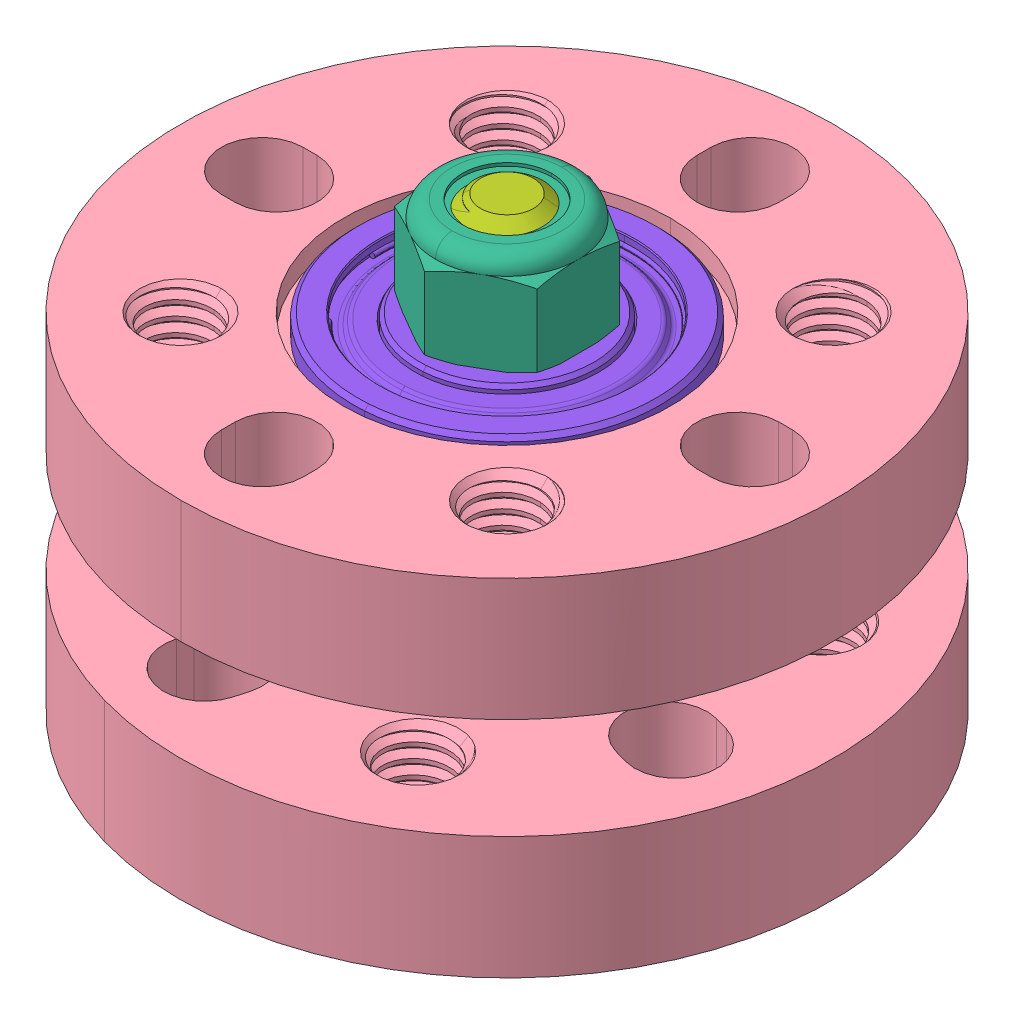
SolidWorks assembly 1608-0001-0001 assembly, configuration Default. Lengths in mm.
Overall size (39.45 26.01 39.45).
22 component instances, 9 part files, 0 mates.
Components (placement in the parent):
- 1608-0001-0001 assembly.STEP-1: 1608-0001-0001 assembly.STEP [Default] at origin size (39.45 26.01 39.45)
  - 1613-0516-0008 assembly.STEP-1: 1613-0516-0008 assembly.STEP [Default] at (13.2242 -21.7608 12.1381) x (0.966093 0 0.258196) z (-0.258196 0 0.966093) size (17.83 4.96 17.83)
    - 1613-0516-0008 carriage.STEP-1: 1613-0516-0008 carriage.STEP [Default] at (-23.0253 -4.8501 14.8236) size (15.72 1.83 15.72)
    - 1613-0516-0008 ball.STEP-1: 1613-0516-0008 ball.STEP [Default] at (-28.8255 -3.9351 16.4353) size (3 3 3)
    - 1613-0516-0008 ball.STEP-2: 1613-0516-0008 ball.STEP [Default] at (-26.4325 -3.9351 19.7866) x (0.766044 0 -0.642788) z (0.642788 0 0.766044) size (3 3 3)
    - 1613-0516-0008 ball.STEP-3: 1613-0516-0008 ball.STEP [Default] at (-22.4452 -3.9351 20.8156) x (0.173648 0 -0.984808) z (0.984808 0 0.173648) size (3 3 3)
    - 1613-0516-0008 ball.STEP-4: 1613-0516-0008 ball.STEP [Default] at (-18.7293 -3.9351 19.0408) x (-0.5 0 -0.866025) z (0.866025 0 -0.5) size (3 3 3)
    - 1613-0516-0008 ball.STEP-5: 1613-0516-0008 ball.STEP [Default] at (-17.0236 -3.9351 15.2928) x (-0.939693 0 -0.34202) z (0.34202 0 -0.939693) size (3 3 3)
    - 1613-0516-0008 ball.STEP-6: 1613-0516-0008 ball.STEP [Default] at (-18.1261 -3.9351 11.3252) x (-0.939693 0 0.34202) z (-0.34202 0 -0.939693) size (3 3 3)
    - 1613-0516-0008 ball.STEP-7: 1613-0516-0008 ball.STEP [Default] at (-21.521 -3.9351 8.9945) x (-0.5 0 0.866025) z (-0.866025 0 -0.5) size (3 3 3)
    - 1613-0516-0008 ball.STEP-8: 1613-0516-0008 ball.STEP [Default] at (-25.6197 -3.9351 9.3913) x (0.173648 0 0.984808) z (-0.984808 0 0.173648) size (3 3 3)
    - 1613-0516-0008 ball.STEP-9: 1613-0516-0008 ball.STEP [Default] at (-28.5045 -3.9351 12.3299) x (0.766044 0 0.642788) z (-0.642788 0 0.766044) size (3 3 3)
    - 1613-0516-0008 washer.STEP-1: 1613-0516-0008 washer.STEP [Default] at (-23.0253 -6.4151 14.8236) size (16 1.28 16)
    - 1613-0516-0008 washer.STEP-2: 1613-0516-0008 washer.STEP [Default] at (-23.0253 -1.4551 14.8236) x (0.992523 0 -0.12206) z (-0.12206 0 -0.992523) size (16 1.28 16)
  - 1504-0032-0060.STEP-1: 1504-0032-0060.STEP [Default] at (-12.8477 -20.2159 20.514) size (31.95 6.01 31.95)
  - 1504-0032-0060.STEP-2: 1504-0032-0060.STEP [Default] at (-12.8477 -31.1759 20.514) x (-0.962134 0 -0.272576) z (-0.272576 0 0.962134) size (31.95 6.01 31.95)
  - 1512-0008-0060.STEP-1: 1512-0008-0060.STEP [Default] at (-12.8477 -26.1759 20.514) x (0.459127 0 -0.888371) z (0.888371 0 0.459127) size (7.95 6 7.95)
  - 2812-0004-0007_90576A103.STEP-1: 2812-0004-0007_90576A103.STEP [Default] at (-12.8477 -17.2659 20.514) size (7.02 4.86 8.1)
  - 2800-0004-0022_90128A207.STEP-1: 2800-0004-0022_90128A207.STEP [Default] at (-12.8477 -12.1759 20.514) x (0.823101 0 -0.567895) z (0 1 0) size (7 7 26.01)
  - 1611-0514-0006.STEP-1: 1611-0514-0006.STEP [Default] at (-12.8477 -22.2159 20.514) x (0.997679 0 -0.068092) z (0.068092 0 0.997679) size (15 5 15)
  - 1611-0514-0006.STEP-2: 1611-0514-0006.STEP [Default] at (-12.8477 -29.1759 20.514) x (-0.139006 0 -0.990292) z (-0.990292 0 0.139006) size (15 5 15)
  - 1502-0006-0165.STEP-1: 1502-0006-0165.STEP [Default] at (-12.8477 -25.9259 20.514) x (0.997115 0 -0.075907) z (0.075907 0 0.997115) size (5.95 16.5 5.95)
